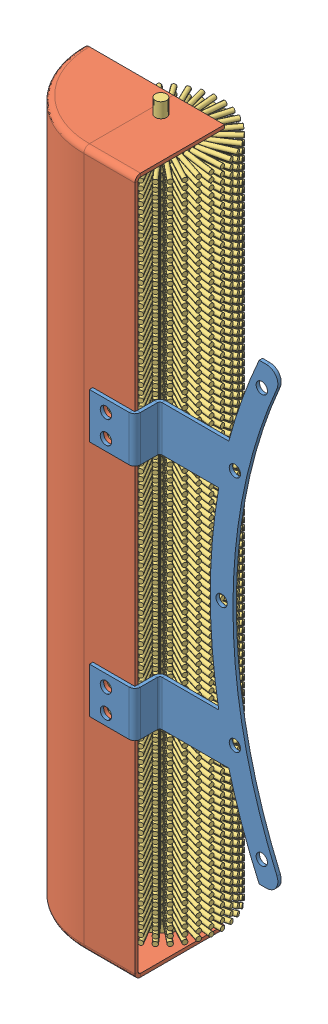
SolidWorks assembly cleaning part, configuration Default. Lengths in mm.
Overall size (115.57 320 56.98).
3 component instances, 3 part files, 5 mates.
Components (placement in the parent):
- holder2-1: holder2 [Default] at (565.4382 75.7061 153.1645) size (72.07 200 12.5)
- Part3-1: Part3 [Default] at (47.6736 218.1083 165.1645) x (-1 0 0) z (0 0 1) size (62 307 39.51)
- brush 2-2: brush 2 [Default] at (24.6736 252.0044 137.1645) x (1 0 0) z (0 -1 0) size (52.04 51.98 320)
Mates (geometry in assembly coordinates):
- Coincident1: coincident anti-aligned: plane of holder2-1 through (565.4382 75.7061 166.6645) normal (0 0 -1); plane of Part3-1 through (47.6736 218.1083 166.6645) normal (0 0 1)
- Coincident2: coincident anti-aligned: plane of holder2-1 through (42.6736 75.7061 153.1645) normal (-1 0 0); plane of Part3-1 through (42.6736 -48.9956 165.1645) normal (1 0 0)
- Concentric2: concentric aligned: circle of holder2-1; circle of Part3-1
- Concentric3: concentric anti-aligned: cylinder of Part3-1 through (24.6736 262.0044 137.1645) axis (0 -1 0) radius 2.5; cylinder of brush 2-2 through (24.6736 -57.9956 137.1645) axis (0 1 0) radius 2.5
- Distance4: distance = 2 mm anti-aligned: plane of brush 2-2 through (24.6736 -47.9956 137.1645) normal (0 -1 0); plane of Part3-1 through (42.6736 -49.9956 165.1645) normal (0 1 0)
